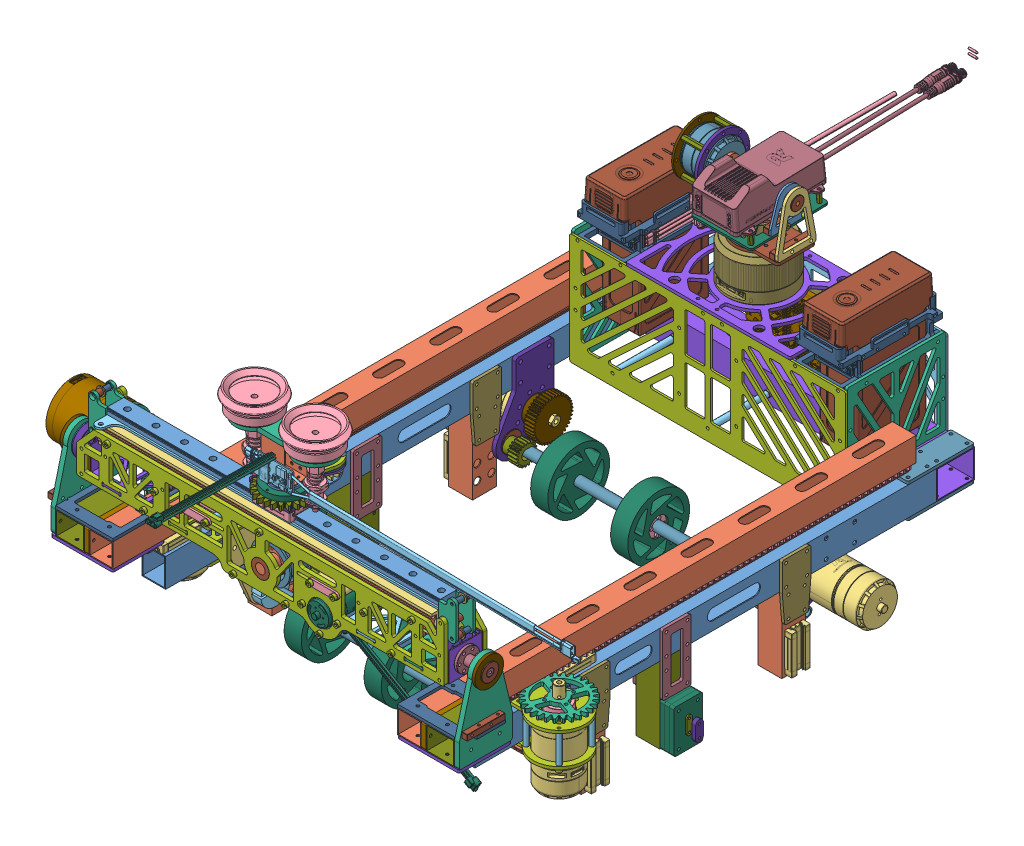
SolidWorks assembly 上层框架总装1.0, configuration 默认. Lengths in mm.
Overall size (616.21 347.11 913.64).
365 component instances, 117 part files, 27 mates.
Components (placement in the parent):
- 前探2.0-1: 前探2.0 [默认] at origin size (502.63 224 581.5) (flexible)
  - 30x25x1铝方管-2: 30x25x1铝方管 [前探底管] at (162.5 0 0) size (25 30 485)
  - 25x25x1铝方管-1: 25x25x1铝方管 [前探长管镜像] at (-162.5 43.5 38) size (25 25 520)
  - 25x25x1铝方管-2: 25x25x1铝方管 [前探长管] at (162.5 43.5 39) size (25 25 520)
  - RoboMaster M3508直流无刷减速电机-1: RoboMaster M3508直流无刷减速电机 [默认] at (-214.3876 -71.441 186.7932) x (0.414106 0 0.910229) z (0 1 0) size (42 42.01 98.4)
  - 推力球轴承-1: 推力球轴承 [51100 10*24*9] at (-198.5 17 177.6) size (24 9 24)
  - 304不锈钢接线柱-1: 304不锈钢接线柱 [M3*30-5] at (-215.8241 0 160.2759) x (0.012605 0 0.999921) z (0 1 0) size (5 5 30)
  - 304不锈钢接线柱-3: 304不锈钢接线柱 [M3*30-5] at (-215.8241 0 194.9241) x (-0.333238 0 0.942843) z (0 1 0) size (5 5 30)
  - 304不锈钢接线柱-4: 304不锈钢接线柱 [M3*30-5] at (-181.1759 0 160.2759) x (-0.333238 0 0.942843) z (0 1 0) size (5 5 30)
  - RoboMaster M3508直流无刷减速电机-2: RoboMaster M3508直流无刷减速电机 [默认] at (207.2166 -71.441 193.754) x (0.922142 0 -0.386852) z (0 1 0) size (42 42.01 98.4)
  - 推力球轴承-2: 推力球轴承 [51100 10*24*9] at (198.5 17 177.6) x (0.998455 0 0.055559) z (-0.055559 0 0.998455) size (24 9 24)
  - 304不锈钢接线柱-5: 304不锈钢接线柱 [M3*30-5] at (215.8241 0 160.2759) x (-0.333238 0 0.942843) z (0 1 0) size (5 5 30)
  - 304不锈钢接线柱-6: 304不锈钢接线柱 [M3*30-5] at (215.8241 0 194.9241) x (-0.333238 0 0.942843) z (0 1 0) size (5 5 30)
  - 304不锈钢接线柱-7: 304不锈钢接线柱 [M3*30-5] at (181.1759 0 194.9241) x (-0.333238 0 0.942843) z (0 1 0) size (5 5 30)
  - 304不锈钢接线柱-8: 304不锈钢接线柱 [M3*30-5] at (181.1759 0 160.2759) x (-0.333238 0 0.942843) z (0 1 0) size (5 5 30)
  - 横移连接板-1: 横移连接板 [电机安装板] at (-210 43.5 263) x (0 0 1) z (-1 0 0) size (101.67 92 5)
  - 12.9级圆柱头螺钉-2: 12.9级圆柱头螺钉 [M3*8] at (-215.8241 -21 194.9241) x (0.053089 0 -0.99859) z (0 -1 0) size (5.68 5.68 11)
  - 12.9级圆柱头螺钉-3: 12.9级圆柱头螺钉 [M3*8] at (-215.8241 -21 160.2759) x (0.053089 0 -0.99859) z (0 -1 0) size (5.68 5.68 11)
  - 12.9级圆柱头螺钉-4: 12.9级圆柱头螺钉 [M3*8] at (-181.1759 -21 160.2759) x (0.998723 0 -0.050526) z (0 -1 0) size (5.68 5.68 11)
  - 12.9级圆柱头螺钉-5: 12.9级圆柱头螺钉 [M3*8] at (181.1759 -21 160.2759) x (0.998723 0 -0.050526) z (0 -1 0) size (5.68 5.68 11)
  - 12.9级圆柱头螺钉-6: 12.9级圆柱头螺钉 [M3*8] at (215.8241 -21 160.2759) x (0.998723 0 -0.050526) z (0 -1 0) size (5.68 5.68 11)
  - 12.9级圆柱头螺钉-7: 12.9级圆柱头螺钉 [M3*8] at (215.8241 -21 194.9241) x (0.998723 0 -0.050526) z (0 -1 0) size (5.68 5.68 11)
  - 12.9级圆柱头螺钉-8: 12.9级圆柱头螺钉 [M3*8] at (181.1759 -21 194.9241) x (0.998723 0 -0.050526) z (0 -1 0) size (5.68 5.68 11)
  - 12.9级圆柱头螺钉-9: 12.9级圆柱头螺钉 [M3*5] at (155 11 230.55) x (0.998723 0 -0.050526) z (0 -1 0) size (5.68 5.68 8)
  - 12.9级圆柱头螺钉-10: 12.9级圆柱头螺钉 [M3*5] at (170 11 230.55) x (0.998723 0 -0.050526) z (0 -1 0) size (5.68 5.68 8)
  - 12.9级圆柱头螺钉-11: 12.9级圆柱头螺钉 [M3*5] at (170 11 214.55) x (0.998723 0 -0.050526) z (0 -1 0) size (5.68 5.68 8)
  - 12.9级圆柱头螺钉-12: 12.9级圆柱头螺钉 [M3*5] at (155 11 214.55) x (0.998723 0 -0.050526) z (0 -1 0) size (5.68 5.68 8)
  - 12.9级圆柱头螺钉-13: 12.9级圆柱头螺钉 [M3*5] at (170 11 140.65) x (0.977106 0 0.212755) z (0 -1 0) size (5.68 5.68 8)
  - 12.9级圆柱头螺钉-16: 12.9级圆柱头螺钉 [M3*5] at (155 11 140.65) x (0.977106 0 0.212755) z (0 -1 0) size (5.68 5.68 8)
  - 12.9级圆柱头螺钉-17: 12.9级圆柱头螺钉 [M3*5] at (170 11 124.65) x (0.177923 0 0.984044) z (0 -1 0) size (5.68 5.68 8)
  - 12.9级圆柱头螺钉-18: 12.9级圆柱头螺钉 [M3*5] at (155 11 124.65) x (0.595095 0 -0.803655) z (0 -1 0) size (5.68 5.68 8)
  - 12.9级圆柱头螺钉-19: 12.9级圆柱头螺钉 [M3*5] at (-155 11 230.55) x (0.978167 0 0.207821) z (0 -1 0) size (5.68 5.68 8)
  - 12.9级圆柱头螺钉-20: 12.9级圆柱头螺钉 [M3*5] at (-170 11 230.55) x (0.999805 0 0.019757) z (0 -1 0) size (5.68 5.68 8)
  - 12.9级圆柱头螺钉-21: 12.9级圆柱头螺钉 [M3*5] at (-155 11 214.55) x (0.980556 0 -0.196239) z (0 -1 0) size (5.68 5.68 8)
  - 12.9级圆柱头螺钉-22: 12.9级圆柱头螺钉 [M3*5] at (-170 11 214.55) x (0.907226 0 -0.420643) z (0 -1 0) size (5.68 5.68 8)
  - 12.9级圆柱头螺钉-23: 12.9级圆柱头螺钉 [M3*5] at (-155 11 140.65) x (0.780533 0 -0.625115) z (0 -1 0) size (5.68 5.68 8)
  - 12.9级圆柱头螺钉-24: 12.9级圆柱头螺钉 [M3*5] at (-170 11 140.65) x (0.620194 0 -0.784448) z (0 -1 0) size (5.68 5.68 8)
  - 12.9级圆柱头螺钉-25: 12.9级圆柱头螺钉 [M3*5] at (-155 11 124.65) x (0.45797 0 -0.888968) z (0 -1 0) size (5.68 5.68 8)
  - 12.9级圆柱头螺钉-26: 12.9级圆柱头螺钉 [M3*5] at (-170 11 124.65) x (0.323869 0 -0.946102) z (0 -1 0) size (5.68 5.68 8)
  - 横移连接板-2: 横移连接板 [转轴转点] at (215 43.5 263) x (0 0 1) z (-1 0 0) size (56 92 5)
  - 支撑连接板-1: 支撑连接板 [右] at (182.5 28 271.5) x (1 0 0) z (0 1 0) size (65 55 3.23)
  - 支撑连接板-2: 支撑连接板 [左] at (-182.5 28 270.5) x (1 0 0) z (0 1 0) size (341.52 580.5 35.52)
  - 4310 减速电机 3D 20221104_defeature-1: 4310 减速电机 3D 20221104_defeature [默认] at (-259 83 224.3345) x (0 -0.998088 0.061814) z (0 0.061814 0.998088) size (56 46 56)
  - 小带轮-1: 小带轮 [主动轮] at (-205.1 83 224.3345) x (1 0 0) z (0 -0.853122 0.521711) size (7 27.19 27.51)
  - 法兰轴承-1: 法兰轴承 [17*26*5-1.1] at (-216.1 83 224.3345) x (0 -0.997676 0.068144) z (0 0.068144 0.997676) size (28 5 28)
  - 4310传动法兰-1: 4310传动法兰 [默认] at (-220 83 224.3345) x (0 0.302939 -0.95301) z (1 0 0) size (33 33 19.9)
  - 小带轮-2: 小带轮 [从动轮] at (-198.1 108 270.5) x (-1 0 0) z (0 -0.971388 -0.237499) size (7 27.19 27.51)
  - 4310安装垫块-1: 4310安装垫块 [默认] at (-215 83 224.3345) x (0 0.536766 0.843731) z (-1 0 0) size (56 56 6) (hidden)
  - 同步带轮挡板-1: 同步带轮挡板 [默认] at (-206.1 83 224.3345) x (0 -0.521711 -0.853122) z (1 0 0) size (30 30 1)
  - 同步带轮挡板-2: 同步带轮挡板 [默认] at (-197.1 83 224.3345) x (0 0.521711 0.853122) z (-1 0 0) size (30 30 1)
  - 同步带轮挡板1-1: 同步带轮挡板1 [默认] at (-197.1 108 270.5) x (0 0.971388 0.237499) z (-1 0 0) size (30 30 1)
  - 同步带轮挡板1-2: 同步带轮挡板1 [默认] at (-206.1 108 270.5) x (0 -0.280014 -0.959996) z (1 0 0) size (30 30 1)
  - 横移转点法兰-1: 横移转点法兰 [默认] at (-193 108 270.5) x (0 0.971388 0.237499) z (-1 0 0) size (22 22 26.1)
  - 25x30x1铝方管-1: 25x30x1铝方管 [前探管] at (-195 43.5 270.5) size (30 25 55)
  - 25x30x1铝方管-2: 25x30x1铝方管 [前探管] at (195 43.5 271.5) size (30 25 55)
  - 法兰轴承-2: 法兰轴承 [8*16*5-1.1] at (-208.9 108 270.5) x (0 -0.454379 0.890809) z (0 -0.890809 -0.454379) size (18 5 18)
  - 法兰轴承-3: 法兰轴承 [8*16*5-1.1] at (208.9 108 270.5) x (0 -0.670714 0.741716) z (0 0.741716 0.670714) size (18 5 18)
  - 同步带1-1: 同步带1 [默认] at (-201.6 108 270.5) x (1 0 0) z (0 0.47619 0.879342) size (6 30.99 83.49)
  - 法兰轴承-4: 法兰轴承 [8*16*5-1.1] at (219.1 108 270.5) x (0 -0.846571 -0.532276) z (0 0.532276 -0.846571) size (18 5 18)
  - 横移转点垫板-1: 横移转点垫板 [默认] at (215 108 270.5) x (0 -0.116472 -0.993194) z (1 0 0) size (30 30 3)
  - 横移转点垫板-2: 横移转点垫板 [默认] at (-218 108 270.5) x (0 0.20708 -0.978324) z (1 0 0) size (30 30 3)
  - 法兰轴承-5: 法兰轴承 [8*16*5-1.1] at (-219.1 108 270.5) x (0 -0.931071 0.364837) z (0 0.364837 0.931071) size (18 5 18)
  - 转点垫片-1: 转点垫片 [默认] at (-219.1 108 270.5) x (0 0.356837 0.934167) z (-1 0 0) size (12 12 2)
  - 转点垫片-2: 转点垫片 [默认] at (221.1 108 270.5) x (0 0.710644 0.703552) z (-1 0 0) size (12 12 2) (hidden)
  - 上银直线导轨线性滑轨MGN-C-O╱MGN-H-O[MGN9H2R475ZACI＋-O]_2-1: 上银直线导轨线性滑轨MGN-C-O╱MGN-H-O[MGN9H2R475ZACI＋-O]_2 [MGN9H-O] at (-162.5 22.8 15.5) x (-1 0 0) z (0 0 1) size (9 6.5 475)
  - 上银直线导轨线性滑轨MGN-C-O╱MGN-H-O[MGN9H2R475ZACI＋-O]_1-1: 上银直线导轨线性滑轨MGN-C-O╱MGN-H-O[MGN9H2R475ZACI＋-O]_1 [MGN9H-O] at (-162.5 22.8 222.55) x (-1 0 0) z (0 0 1) size (20 7.8 39.98)
  - 上银直线导轨线性滑轨MGN-C-O╱MGN-H-O[MGN9H2R475ZACI＋-O]_1-2: 上银直线导轨线性滑轨MGN-C-O╱MGN-H-O[MGN9H2R475ZACI＋-O]_1 [MGN9H-O] at (-162.5 22.8 132.65) x (-1 0 0) z (0 0 1) size (20 7.8 39.98)
  - 30x25x1铝方管-6: 30x25x1铝方管 [前探底管] at (-162.5 0 0) size (25 30 485)
  - 上银直线导轨线性滑轨MGN-C-O╱MGN-H-O[MGN9H2R475ZACI＋-O]_2-2: 上银直线导轨线性滑轨MGN-C-O╱MGN-H-O[MGN9H2R475ZACI＋-O]_2 [MGN9H-O] at (162.5 22.8 16.5) x (-1 0 0) z (0 0 1) size (9 6.5 475)
  - 上银直线导轨线性滑轨MGN-C-O╱MGN-H-O[MGN9H2R475ZACI＋-O]_1-3: 上银直线导轨线性滑轨MGN-C-O╱MGN-H-O[MGN9H2R475ZACI＋-O]_1 [MGN9H-O] at (162.5 22.8 222.55) x (-1 0 0) z (0 0 1) size (20 7.8 39.98)
  - 上银直线导轨线性滑轨MGN-C-O╱MGN-H-O[MGN9H2R475ZACI＋-O]_1-4: 上银直线导轨线性滑轨MGN-C-O╱MGN-H-O[MGN9H2R475ZACI＋-O]_1 [MGN9H-O] at (162.5 22.8 132.65) x (-1 0 0) z (0 0 1) size (20 7.8 39.98)
  - 齿条2X76-1: 齿条2X76 [默认] at (168 31 244) x (0 0 -1) z (0 -1 0) size (465 14.5 6)
  - 齿条2X76-3: 齿条2X76 [默认] at (-168 25 243) x (0 0 -1) z (0 1 0) size (465 14.5 6)
  - 2孔夹紧联轴器-1: 2孔夹紧联轴器 [默认] at (-198.5 30 177.6) x (-0.289177 0 0.957276) z (0 1 0) size (28 32 12)
  - 3508前探电机安装板-3: 3508前探电机安装板 [默认] at (-225 19 185.3862) x (0 0 1) z (0 -1 0) size (80 120 0)
  - 圆柱齿轮28×2-1: 圆柱齿轮28×2 [默认] at (-198.5 30 177.6) x (0.942893 0 0.333096) z (0 -1 0) size (59.77 59.77 4)
  - 前探3508安装板-1: 前探3508安装板 [3508安装板] at (-198.5 16.5 177.6) x (0 0 -1) z (0 1 0) size (55 76 3)
  - 2孔夹紧联轴器-2: 2孔夹紧联轴器 [默认] at (198.5 30 177.6) x (-0.289177 0 0.957276) z (0 1 0) size (28 32 12) (hidden)
  - 圆柱齿轮28×2-2: 圆柱齿轮28×2 [默认] at (198.5 30 177.6) x (0.942893 0 0.333096) z (0 -1 0) size (59.77 59.77 4)
  - 前探3508安装板-2: 前探3508安装板 [3508安装板] at (198.5 16.5 177.6) x (0 0 -1) z (0 -1 0) size (55 76 3)
  - 40x30x1铝方管-1: 40x30x1铝方管 [默认] at (0 0 -262.5) x (0 0 1) z (-1 0 0) size (40 30 350)
  - 前探3508安装板-3: 前探3508安装板 [下端固定板] at (-198.5 -16.5 177.6) x (0 0 -1) z (0 1 0) size (55 76 3)
  - 304不锈钢接线柱-9: 304不锈钢接线柱 [M3*30-5] at (-181.1759 0 194.9241) x (-0.440055 0 0.897971) z (0 1 0) size (5 5 30)
  - 12.9级圆柱头螺钉-27: 12.9级圆柱头螺钉 [M3*8] at (-181.1759 -21 194.9241) x (-0.034714 0 -0.999397) z (0 -1 0) size (5.68 5.68 11)
  - 前探3508安装板-4: 前探3508安装板 [下端固定板] at (198.5 -16.5 177.6) x (0 0 -1) z (0 -1 0) size (55 76 3)
  - 25x25x1铝方管-3: 25x25x1铝方管 [抬升滑块安装管] at (162.5 -55 118.4) x (1 0 0) z (0 -1 0) size (25 25 80)
  - 25x25x1铝方管-4: 25x25x1铝方管 [抬升滑块安装管] at (162.5 -55 -92.4) x (1 0 0) z (0 -1 0) size (25 25 80)
  - 上银直线导轨线性滑轨MGN-C-O╱MGN-H-O[MGN9H2R475ZACI＋-O]_1-5: 上银直线导轨线性滑轨MGN-C-O╱MGN-H-O[MGN9H2R475ZACI＋-O]_1 [MGN9H-O] at (182.8 -72.05 118.4) x (0 0 -1) z (0 1 0) size (20 7.8 39.98)
  - 上银直线导轨线性滑轨MGN-C-O╱MGN-H-O[MGN9H2R475ZACI＋-O]_1-6: 上银直线导轨线性滑轨MGN-C-O╱MGN-H-O[MGN9H2R475ZACI＋-O]_1 [MGN9H-O] at (182.8 -72.05 -92.4) x (0 0 -1) z (0 1 0) size (20 7.8 39.98)
  - 25x25x1铝方管-5: 25x25x1铝方管 [抬升滑块安装管] at (-162.5 -55 118.4) x (-1 0 0) z (0 -1 0) size (25 25 80)
  - 25x25x1铝方管-6: 25x25x1铝方管 [抬升滑块安装管] at (-162.5 -55 -92.4) x (-1 0 0) z (0 -1 0) size (25 25 80)
  - 上银直线导轨线性滑轨MGN-C-O╱MGN-H-O[MGN9H2R475ZACI＋-O]_1-7: 上银直线导轨线性滑轨MGN-C-O╱MGN-H-O[MGN9H2R475ZACI＋-O]_1 [MGN9H-O] at (-182.8 -72.05 -92.4) x (0 0 -1) z (0 -1 0) size (20 7.8 39.98)
  - 上银直线导轨线性滑轨MGN-C-O╱MGN-H-O[MGN9H2R475ZACI＋-O]_1-8: 上银直线导轨线性滑轨MGN-C-O╱MGN-H-O[MGN9H2R475ZACI＋-O]_1 [MGN9H-O] at (-182.8 -72.05 118.4) x (0 0 -1) z (0 -1 0) size (20 7.8 39.98)
  - 前探垫块-1: 前探垫块 [默认] at (-180 43.5 270.5) x (0 0 -1) z (1 0 0) size (55 25 5)
  - 前探垫块-2: 前探垫块 [默认] at (175 43.5 271.5) x (0 0 -1) z (1 0 0) size (55 25 5)
  - 前探加固板-1: 前探加固板 [默认] at (-180 59 270.5) x (0 0 1) z (0 -1 0) size (55 71 3)
  - 四孔直角转接件-1: 四孔直角转接件 [上交角件] at (-218 62 275.5) x (0 1 0) z (0 0 1) size (6 6 40)
  - 前探加固板-2: 前探加固板 [默认] at (180 56 271.5) x (0 0 1) z (0 1 0) size (55 71 3)
  - 四孔直角转接件-2: 四孔直角转接件 [上交角件] at (218 62 276.5) x (0 1 0) z (0 0 1) size (6 6 40)
  - 25x30x1铝方管-3: 25x30x1铝方管 [抬升管] at (-162.5 -55 33.295) x (0 0 1) z (0 1 0) size (30 25 80)
  - 25x30x1铝方管-4: 25x30x1铝方管 [抬升管] at (162.5 -55 33.295) x (0 0 -1) z (0 1 0) size (30 25 80)
  - 抬升连接板1-1: 抬升连接板1 [默认] at (-176.5 0 -92.4) x (0 0 1) z (-1 0 0) size (30 60 3)
  - 抬升连接板1-2: 抬升连接板1 [默认] at (-176.5 0 118.4) x (0 0 -1) z (1 0 0) size (30 60 3)
  - 抬升连接板1-3: 抬升连接板1 [默认] at (-148.5 0 -92.4) x (0 0 1) z (-1 0 0) size (30 60 3)
  - 抬升连接板1-4: 抬升连接板1 [默认] at (-148.5 0 118.4) x (0 0 -1) z (1 0 0) size (30 60 3)
  - 抬升连接板2-1: 抬升连接板2 [默认] at (-175 -17.5 33.295) x (0 0 1) z (-1 0 0) size (30 65 3)
  - 抬升连接板2-2: 抬升连接板2 [默认] at (-147 -17.5 33.295) x (0 0 1) z (-1 0 0) size (30 65 3)
  - 抬升连接板1-5: 抬升连接板1 [默认] at (176.5 0 118.4) x (0 0 -1) z (1 0 0) size (30 60 3)
  - 抬升连接板1-6: 抬升连接板1 [默认] at (148.5 0 118.4) x (0 0 -1) z (1 0 0) size (30 60 3)
  - 抬升连接板1-7: 抬升连接板1 [默认] at (176.5 0 -92.4) x (0 0 -1) z (1 0 0) size (30 60 3)
  - 抬升连接板1-8: 抬升连接板1 [默认] at (148.5 0 -92.4) x (0 0 -1) z (1 0 0) size (30 60 3)
  - 抬升连接板2-3: 抬升连接板2 [默认] at (178 -17.5 33.295) x (0 0 1) z (-1 0 0) size (30 65 3)
  - 抬升连接板2-4: 抬升连接板2 [默认] at (150 -17.5 33.295) x (0 0 1) z (-1 0 0) size (30 65 3)
  - 前探连接板-1: 前探连接板 [默认] at (-162.5 15 -247.5) x (0 0 -1) z (0 1 0) size (70 25 3)
  - 前探连接板-2: 前探连接板 [默认] at (162.5 15 -247.5) x (0 0 -1) z (0 1 0) size (70 25 3)
  - 前探连接板-3: 前探连接板 [默认] at (162.5 -18 -247.5) x (0 0 -1) z (0 1 0) size (70 25 3)
  - 前探连接板-4: 前探连接板 [默认] at (-162.5 -18 -247.5) x (0 0 -1) z (0 1 0) size (70 25 3)
  - 抬升链条连接-1: 抬升链条连接 [底层] at (-175 -72.5 33.295) x (0 0 1) z (-1 0 0) size (30 45 5)
  - 抬升链条连接-2: 抬升链条连接 [二层] at (-180 -72.5 33.295) x (0 0 1) z (-1 0 0) size (30 45 5)
  - 抬升链条连接-5: 抬升链条连接 [连接一层] at (-185 -72.5 33.295) x (0 0 1) z (-1 0 0) size (30 45 5)
  - 链条连接垫块-1: 链条连接垫块 [默认] at (-190 -72.5 33.295) x (0 0 1) z (-1 0 0) size (6 18.7 1.31)
  - 链条连接-1: 链条连接 [默认] at (-197.69 -72.5 33.295) x (0 0 1) z (-1 0 0) size (8 20.7 4)
  - 抬升链条连接-6: 抬升链条连接 [底层] at (180 -72.5 33.295) x (0 0 1) z (-1 0 0) size (30 45 5)
  - 抬升链条连接-8: 抬升链条连接 [底层] at (185 -72.5 33.295) x (0 0 1) z (-1 0 0) size (30 45 5)
  - 抬升链条连接-9: 抬升链条连接 [连接一层] at (190 -72.5 33.295) x (0 0 1) z (-1 0 0) size (30 45 5)
  - 链条连接垫块-2: 链条连接垫块 [默认] at (191.31 -72.5 33.295) x (0 0 1) z (-1 0 0) size (6 18.7 1.31)
  - 链条连接-2: 链条连接 [默认] at (201.69 -72.5 33.295) x (0 0 1) z (-1 0 0) size (8 20.7 4)
- 取矿横移总装-1: 取矿横移总装 [默认] at (0 138 270.5) x (0 0 -1) z (1 0 0) size (203.34 276.76 526.28)
  - 横移总装2.0-1: 横移总装2.0 [默认] at origin size (67.7 199.63 415.26)
    - 20x20x1铝方管-1: 20x20x1铝方管 [默认] at (0 2.5 0.2898) size (15 15 350)
    - 上银直线导轨线性滑轨MGW-C╱MGW-H[MGW9C2R355EZACHCI]_2-1: 上银直线导轨线性滑轨MGW-C╱MGW-H[MGW9C2R355EZACHCI]_2 [横移] at (0 14.9 0.2898) size (18 7 350)
    - 铝合金抽屉滑轨_350-1: 铝合金抽屉滑轨_350 [默认] at (12.9 0 0) x (0 0 -1) z (-1 0 0) size (350.29 20 8) (flexible)
      - 铝合金抽屉滑轨内侧_350-1: 铝合金抽屉滑轨内侧_350 [默认] at origin size (350 12 5.6)
      - 铝合金抽屉滑轨外侧_350-1: 铝合金抽屉滑轨外侧_350 [默认] at (-0.2898 0 2.4) size (350 20 7.2)
    - 铝合金抽屉滑轨_350-2: 铝合金抽屉滑轨_350 [默认] at (-12.9 0 0) x (0 0 -1) z (1 0 0) size (350.29 20 8) (flexible)
      - 铝合金抽屉滑轨内侧_350-1: 铝合金抽屉滑轨内侧_350 [默认] at origin size (350 12 5.6)
      - 铝合金抽屉滑轨外侧_350-1: 铝合金抽屉滑轨外侧_350 [默认] at (-0.2898 0 2.4) size (350 20 7.2)
    - 上银直线导轨线性滑轨MGW-C╱MGW-H[MGW9C2R355EZACHCI]_1-1: 上银直线导轨线性滑轨MGW-C╱MGW-H[MGW9C2R355EZACHCI]_1 [MGW9C] at (0 14.9 3.3555) size (30 9.1 39.49)
    - 滑轨安装板-1: 滑轨安装板 [默认] at (0 10 0.2898) x (0 0 -1) z (0 1 0) size (350 50.5 2)
    - 转点安装板1-1: 转点安装板1 [默认] at (7.5 2.5 160.2898) x (0 0 -1) z (1 0 0) size (48 39.5 3)
    - 转点安装板1-2: 转点安装板1 [默认] at (-10.5 2.5 160.2898) x (0 0 -1) z (1 0 0) size (48 39.5 3)
    - 转点安装板1-3: 转点安装板1 [默认] at (10.5 2.5 -159.7102) x (0 0 1) z (-1 0 0) size (48 39.5 3)
    - 转点安装板1-4: 转点安装板1 [默认] at (-7.5 2.5 -159.7102) x (0 0 1) z (-1 0 0) size (48 39.5 3)
    - 安装固定板-2: 安装固定板 [非2006安装板] at (-22.5 -20 0) x (0 0 -1) z (1 0 0) size (386 79.31 4)
    - 35x10x1铝方管-1: 35x10x1铝方管 [默认] at (0 -30 188) x (1 0 0) z (0 -1 0) size (35 10 30)
    - 垫板-1: 垫板 [默认] at (-18 -30 188) x (0 0 1) z (-1 0 0) size (10 30 1)
    - 垫板-2: 垫板 [默认] at (18 -30 188) x (0 0 1) z (-1 0 0) size (10 30 1)
    - 35x10x1铝方管-2: 35x10x1铝方管 [默认] at (0 -30 -188) x (1 0 0) z (0 -1 0) size (35 10 30)
    - 垫板-3: 垫板 [默认] at (-18 -30 -188) x (0 0 1) z (-1 0 0) size (10 30 1)
    - 垫板-4: 垫板 [默认] at (18 -30 -188) x (0 0 1) z (-1 0 0) size (10 30 1)
    - 鸿康明铝柱-1: 鸿康明铝柱 [M3*8] at (-3.5 22.5 189.2898) x (1 0 0) z (0 -0.954265 0.298963) size (8 5 5)
    - 粉末冶金铜套-1: 粉末冶金铜套 [默认] at (4.5 22.5 189.2898) x (0 0.169784 0.985481) z (-1 0 0) size (6 6 6)
    - 3x9x1垫片-1: 3x9x1垫片 [默认] at (1 22.5 189.2898) x (0 -0.61264 -0.790362) z (1 0 0) size (9 9 1)
    - 鸿康明铝柱-2: 鸿康明铝柱 [M3*8] at (-3.5 -2.5 180.2898) x (1 0 0) z (0 -0.617564 0.786521) size (8 5 5)
    - 粉末冶金铜套-2: 粉末冶金铜套 [默认] at (4.5 -2.5 180.2898) x (0 -0.015386 0.999882) z (-1 0 0) size (6 6 6)
    - 3x9x1垫片-2: 3x9x1垫片 [默认] at (1 -2.5 180.2898) x (0 -0.61264 -0.790362) z (1 0 0) size (9 9 1)
    - 粉末冶金铜套-3: 粉末冶金铜套 [默认] at (-4.5 -9 189.2898) x (0 -0.015317 0.999883) z (-1 0 0) size (6 6 6)
    - 鸿康明铝柱-3: 鸿康明铝柱 [M3*8] at (3.5 -9 189.2898) x (1 0 0) z (0 -0.94021 0.340594) size (8 5 5)
    - 3x9x1垫片-3: 3x9x1垫片 [默认] at (-1 -9 189.2898) x (0 -0.634328 -0.773064) z (1 0 0) size (9 9 1)
    - 鸿康明铝柱-4: 鸿康明铝柱 [M3*8] at (3.5 22.5 -188.7102) x (1 0 0) z (0 -0.954265 0.298963) size (8 5 5)
    - 粉末冶金铜套-4: 粉末冶金铜套 [默认] at (-4.5 22.5 -188.7102) x (0 0.169784 0.985481) z (-1 0 0) size (6 6 6)
    - 3x9x1垫片-4: 3x9x1垫片 [默认] at (-1 22.5 -188.7102) x (0 -0.708763 -0.705447) z (1 0 0) size (9 9 1)
    - 鸿康明铝柱-5: 鸿康明铝柱 [M3*8] at (3.5 -2.5 -179.7102) x (1 0 0) z (0 -0.919061 0.394116) size (8 5 5)
    - 粉末冶金铜套-5: 粉末冶金铜套 [默认] at (-4.5 -2.5 -179.7102) x (0 0.138586 0.99035) z (-1 0 0) size (6 6 6)
    - 3x9x1垫片-5: 3x9x1垫片 [默认] at (-1 -2.5 -179.7102) x (0 -0.708763 -0.705447) z (1 0 0) size (9 9 1)
    - 鸿康明铝柱-6: 鸿康明铝柱 [M3*8] at (-3.5 -9 -188.7102) x (1 0 0) z (0 -0.453676 0.891166) size (8 5 5)
    - 3x9x1垫片-6: 3x9x1垫片 [默认] at (1 -9 -188.7102) x (0 -0.708763 -0.705447) z (1 0 0) size (9 9 1)
    - 粉末冶金铜套-6: 粉末冶金铜套 [默认] at (4.5 -9 -188.7102) x (0 0.138586 0.99035) z (-1 0 0) size (6 6 6)
    - 深沟球轴承-1: 深沟球轴承 [3x7x3] at (15.2 -13.5 163) x (0 -0.844681 -0.53527) z (0 -0.53527 0.844681) size (7 3 7)
    - 深沟球轴承-2: 深沟球轴承 [3x7x3] at (15.2 0.4813 104.6517) x (0 -0.771668 0.636026) z (0 0.636026 0.771668) size (7 3 7)
    - 深沟球轴承-3: 深沟球轴承 [3x7x3] at (15.2 -13.5 -103) x (0 -0.533975 -0.845501) z (0 -0.845501 0.533975) size (7 3 7)
    - 深沟球轴承-4: 深沟球轴承 [3x7x3] at (15.2 -13.5 -163) x (0 0.004458 -0.99999) z (0 -0.99999 -0.004458) size (7 3 7)
    - 深沟球轴承-5: 深沟球轴承 [3x7x3] at (-18.2 -13.5 163) x (0 -0.963854 -0.266431) z (0 -0.266431 0.963854) size (7 3 7)
    - 深沟球轴承-6: 深沟球轴承 [3x7x3] at (-18.2 -13.5 103) x (0 0.996588 0.082533) z (0 0.082533 -0.996588) size (7 3 7)
    - 深沟球轴承-7: 深沟球轴承 [3x7x3] at (-18.2 -13.5 -103) x (0 -0.057804 -0.998328) z (0 -0.998328 0.057804) size (7 3 7)
    - 深沟球轴承-8: 深沟球轴承 [3x7x3] at (-18.2 -13.5 -163) x (0 -0.915157 -0.403098) z (0 -0.403098 0.915157) size (7 3 7)
    - 铰轮1.0-1: 铰轮1.0 [默认] at (0 -34 0) x (0 0.984367 0.176128) z (0 -0.176128 0.984367) size (41 24 41)
    - 法兰轴承-1: 法兰轴承 [10*19*5-1] at (17.5 -34 0) x (0 -0.704143 0.710058) z (0 0.710058 0.704143) size (21 5 21)
    - RoboMaster M2006 P36直流无刷减速电机-1: RoboMaster M2006 P36直流无刷减速电机 [默认] at (-11.3952 -31.5927 46.0167) x (0 -0.258819 -0.965926) z (-1 0 0) size (140.17 141.41 64.8)
    - 安装固定板-3: 安装固定板 [2006安装板] at (18.5 -20 0) x (0 0 -1) z (1 0 0) size (386 79.31 4)
    - 小带轮3Mx25-1: 小带轮3Mx25 [默认] at (25.4 -42.8 63.1397) x (1 0 0) z (0 -0.934457 -0.356076) size (6 23.05 23.09)
    - 大带轮3Mx50-1: 大带轮3Mx50 [默认] at (25.4 -34 0) x (1 0 0) z (0 0.986511 0.163695) size (6 46.93 46.99)
    - 推力球轴承-1: 推力球轴承 [F6-12M 6*12*4] at (24.4 -42.8 63.1397) x (0 0.637207 0.770693) z (0 -0.770693 0.637207) size (12 4 12)
    - 小带轮挡边-1: 小带轮挡边 [默认] at (25.4 -42.8 63.1397) x (0 0.491726 0.87075) z (-1 0 0) size (26 26 1)
    - 小带轮挡边-2: 小带轮挡边 [默认] at (32.4 -42.8 63.1397) x (0 0.997033 0.076981) z (-1 0 0) size (26 26 1)
    - 大带轮挡边-1: 大带轮挡边 [默认] at (32.4 -34 0) x (0 -0.163695 0.986511) z (-1 0 0) size (56 56 1)
    - 大带轮挡边-2: 大带轮挡边 [默认] at (25.4 -34 0) x (0 -0.163695 0.986511) z (-1 0 0) size (56 56 1)
    - 法兰轴承-2: 法兰轴承 [10*19*5-1] at (-17.5 -34 0) x (0 0.968123 0.250476) z (0 -0.250476 0.968123) size (21 5 21)
    - 传动轴-1: 传动轴 [默认] at (-22.5 -34 0) x (0 -0.984367 -0.176128) z (-1 0 0) size (24 24 60.8)
    - 鸿康明铝柱-7: 鸿康明铝柱 [M3*37] at (0 -18 110) size (37 5 5)
    - 鸿康明铝柱-8: 鸿康明铝柱 [M3*37] at (0 -18 -110) size (37 5 5)
    - 槽轮安装件-1: 槽轮安装件 [默认] at (-5 -18 67.5) x (0 0 1) z (0 1 0) size (32 23 7)
    - 槽轮安装件-2: 槽轮安装件 [默认] at (5 -18 -67.5) x (0 0 -1) z (0 1 0) size (32 23 7)
    - 垫片安装-1: 垫片安装 [默认] at (17.5 -18 -67.5) x (0 0 -1) z (1 0 0) size (32 7 2)
    - 垫片安装-2: 垫片安装 [默认] at (-7.5 -18 -67.5) x (0 0 -1) z (1 0 0) size (32 7 2)
    - 垫片安装-3: 垫片安装 [默认] at (-23.5 -18 -67.5) x (0 0 -1) z (1 0 0) size (32 7 2)
    - 304不锈钢接线柱-1: 304不锈钢接线柱 [M3*10-6] at (-13.5 -18 -80) x (0 0.392513 0.919746) z (-1 0 0) size (6 6 10)
    - 304不锈钢接线柱-2: 304不锈钢接线柱 [M3*10-6] at (-13.5 -18 -55) x (0 0.520007 0.854162) z (-1 0 0) size (6 6 10)
    - 垫片安装-4: 垫片安装 [默认] at (23.5 -18 -67.5) x (0 0 -1) z (1 0 0) size (32 7 2)
    - 垫片安装-5: 垫片安装 [默认] at (-17.5 -18 67.5) x (0 0 -1) z (1 0 0) size (32 7 2)
    - 垫片安装-6: 垫片安装 [默认] at (7.5 -18 67.5) x (0 0 -1) z (1 0 0) size (32 7 2)
    - 垫片安装-7: 垫片安装 [默认] at (23.5 -18 67.5) x (0 0 -1) z (1 0 0) size (32 7 2)
    - 垫片安装-8: 垫片安装 [默认] at (-23.5 -18 67.5) x (0 0 -1) z (1 0 0) size (32 7 2)
    - 304不锈钢接线柱-3: 304不锈钢接线柱 [M3*10-6] at (13.5 -18 80) x (0 0.51626 0.856432) z (-1 0 0) size (6 6 10)
    - 304不锈钢接线柱-4: 304不锈钢接线柱 [M3*10-6] at (13.5 -18 55) x (0 0.48843 0.872603) z (-1 0 0) size (6 6 10)
    - 鸿康明铝柱-9: 鸿康明铝柱 [M3*37] at (0 -41 138.7695) size (37 5 5)
    - 鸿康明铝柱-10: 鸿康明铝柱 [M3*37] at (0 -42.8 81.6519) size (37 5 5)
    - 鸿康明铝柱-11: 鸿康明铝柱 [M3*37] at (0 -61.3122 63.1397) size (37 5 5)
    - 鸿康明铝柱-12: 鸿康明铝柱 [M3*37] at (0 -42.8 44.6275) size (37 5 5)
    - 鸿康明铝柱-13: 鸿康明铝柱 [M3*37] at (0 -52 27.5) size (37 5 5)
    - 鸿康明铝柱-14: 鸿康明铝柱 [M3*37] at (0 -52 -27.5) size (37 5 5)
    - 鸿康明铝柱-16: 鸿康明铝柱 [M3*37] at (0 -41 -121.5) x (1 0 0) z (0 -0.672533 0.740067) size (37 5 5)
    - 加强板1-1: 加强板1 [默认] at (0 -39 110.5695) x (0 0 -1) z (0 -1 0) size (50 45 2)
    - 加强板2-1: 加强板2 [默认] at (0 -41 161.9695) x (1 0 0) z (0 1 0) size (45 40 2)
    - 加强板3-1: 加强板3 [默认] at (0 -41 -85.8) x (0 0 1) z (-1 0 0) size (65 2 45)
    - 加强板4-1: 加强板4 [默认] at (0 -41 -153.2) x (0 0 1) z (-1 0 0) size (57 2 45)
    - 2006D型孔联轴器-1: 2006D型孔联轴器 [默认] at (35.4 -42.8 63.1397) x (0 0.844273 0.535914) z (-1 0 0) size (19.05 22 6)
    - V型轴承623zz-1: V型轴承623zz [默认] at (4 -18 55) x (1 0 0) z (0 -0.119134 0.992878) size (3.8 12 12)
    - V型轴承623zz-2: V型轴承623zz [默认] at (-4 -18 -55) x (1 0 0) z (0 -0.119134 0.992878) size (3.8 12 12)
    - 夹紧连轴器-1: 夹紧连轴器 [默认] at (35.4 -34 0) x (0 0.176128 -0.984367) z (1 0 0) size (30.94 31 6)
    - 12.9级圆柱头螺钉-1: 12.9级圆柱头螺钉 [M3*10] at (25.5 -41 138.7695) x (0 -0.265301 -0.964166) z (1 0 0) size (5.68 5.68 13)
    - 12.9级圆柱头螺钉-2: 12.9级圆柱头螺钉 [M3*10] at (25.5 -18 110) x (0 -0.265301 -0.964166) z (1 0 0) size (5.68 5.68 13)
    - 12.9级圆柱头螺钉-3: 12.9级圆柱头螺钉 [M3*10] at (25.5 -42.8 81.6519) x (0 -0.265301 -0.964166) z (1 0 0) size (5.68 5.68 13)
    - 12.9级圆柱头螺钉-4: 12.9级圆柱头螺钉 [M3*10] at (27.5 -18 80) x (0 -0.265301 -0.964166) z (1 0 0) size (5.68 5.68 13)
    - 12.9级圆柱头螺钉-5: 12.9级圆柱头螺钉 [M3*10] at (27.5 -18 55) x (0 -0.265301 -0.964166) z (1 0 0) size (5.68 5.68 13)
    - 12.9级圆柱头螺钉-6: 12.9级圆柱头螺钉 [M3*10] at (25.5 -61.3122 63.1397) x (0 -0.265301 -0.964166) z (1 0 0) size (5.68 5.68 13)
    - 12.9级圆柱头螺钉-8: 12.9级圆柱头螺钉 [M3*10] at (25.5 -52 -27.5) x (0 -0.265301 -0.964166) z (1 0 0) size (5.68 5.68 13)
    - 12.9级圆柱头螺钉-9: 12.9级圆柱头螺钉 [M3*10] at (27.5 -18 -55) x (0 -0.265301 -0.964166) z (1 0 0) size (5.68 5.68 13)
    - 12.9级圆柱头螺钉-10: 12.9级圆柱头螺钉 [M3*10] at (27.5 -18 -80) x (0 -0.265301 -0.964166) z (1 0 0) size (5.68 5.68 13)
    - 12.9级圆柱头螺钉-11: 12.9级圆柱头螺钉 [M3*10] at (25.5 -18 -110) x (0 -0.265301 -0.964166) z (1 0 0) size (5.68 5.68 13)
    - 12.9级圆柱头螺钉-12: 12.9级圆柱头螺钉 [M3*10] at (25.5 -41 -121.5) x (0 -0.265301 -0.964166) z (1 0 0) size (5.68 5.68 13)
    - 12.9级圆柱头螺钉-13: 12.9级圆柱头螺钉 [M3*10] at (-25.5 -41 -121.5) x (0 -0.999995 -0.003259) z (-1 0 0) size (5.68 5.68 13)
    - 12.9级圆柱头螺钉-14: 12.9级圆柱头螺钉 [M3*10] at (-25.5 -18 -110) x (0 -0.999995 -0.003259) z (-1 0 0) size (5.68 5.68 13)
